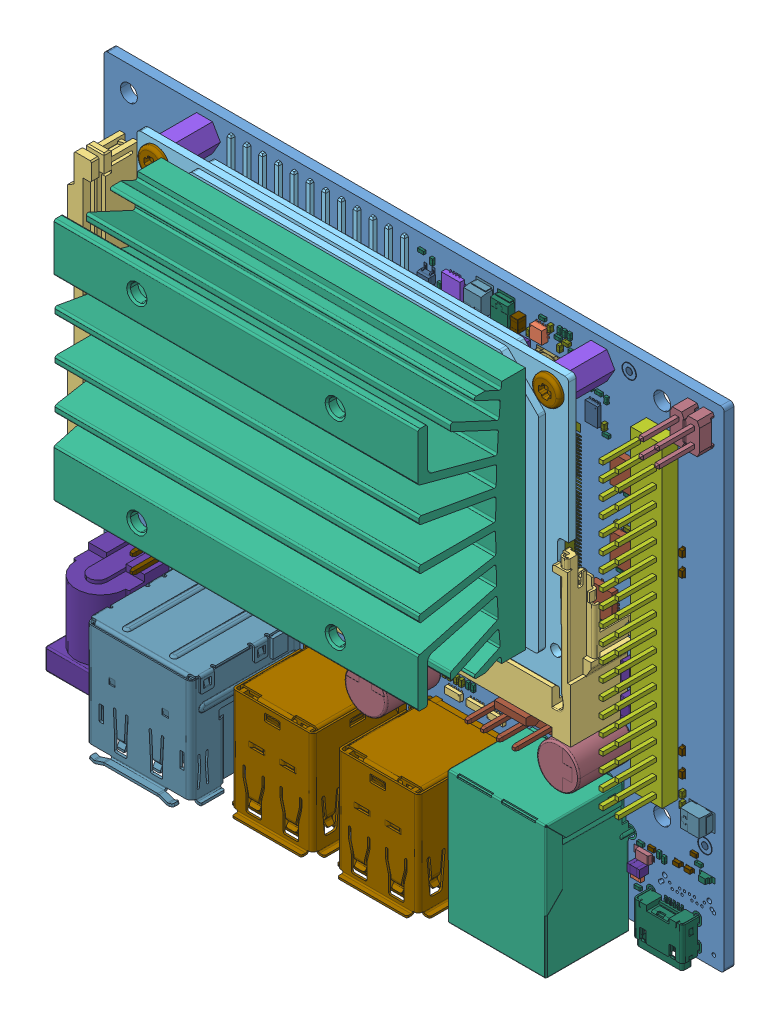
SolidWorks assembly Jetson_Nano_Dev_Kit_3D_b01, configuration Default. Lengths in mm. (continued)
Components (placement in the parent): (continued)
- Jetson_Nano_Dev_Kit_3D_b01(2)^Jetson_Nano_Dev_Kit_3D_b01-1: Jetson_Nano_Dev_Kit_3D_b01(2)^Jetson_Nano_Dev_Kit_3D_b01 [Default] at origin size (100 81.03 30.51) (virtual) (continued)
  - 642-13450_PORG_SYS_BOM^Jetson_Nano_Dev_Kit_3D_b01(2)_Jetson_Nano_Dev_Kit_3D_b01-1: 642-13450_PORG_SYS_BOM^Jetson_Nano_Dev_Kit_3D_b01(2)_Jetson_Nano_Dev_Kit_3D_b01 [Default] at origin size (100 81.03 23.18) (virtual) (continued)
    - 699-13449_PORG_DEV_KIT_PCB_ASSY^642-13450_PORG_SYS_BOM_Jetson_Nano_Dev_Kit_3D_b01(2)_Jetson_Nano_Dev_Kit_3D_b01-1: 699-13449_PORG_DEV_KIT_PCB_ASSY^642-13450_PORG_SYS_BOM_Jetson_Nano_Dev_Kit_3D_b01(2)_Jetson_Nano_Dev_Kit_3D_b01 [Default] at origin size (100 81.03 23.18) (virtual) (continued)
      - 600-13449_PORG_DEV_KIT_PCB_ASSY^699-13449_PORG_DEV_KIT_PCB_ASSY_642-13450_PORG_SYS_BOM_Jetson_Nano_Dev_Kit_3D_b01(2)_Jetson_Nano_Dev_Kit_3D_b01-1: 600-13449_PORG_DEV_KIT_PCB_ASSY^699-13449_PORG_DEV_KIT_PCB_ASSY_642-13450_PORG_SYS_BOM_Jetson_Nano_Dev_Kit_3D_b01(2)_Jetson_Nano_Dev_Kit_3D_b01 [Default] at origin size (100 81.03 23.18) (virtual) (continued)
        - 142-13449-1000-B01-SKU0000^600-13449_PORG_DEV_KIT_PCB_ASSY_699-13449_PORG_DEV_KIT_PCB_ASSY_642-13450_PORG_SYS_BOM_Jetson_Nano_Dev_Kit_3D_b01(2)_Jetson_Nano_Dev_Kit_3D_b01-1: 142-13449-1000-B01-SKU0000^600-13449_PORG_DEV_KIT_PCB_ASSY_699-13449_PORG_DEV_KIT_PCB_ASSY_642-13450_PORG_SYS_BOM_Jetson_Nano_Dev_Kit_3D_b01(2)_Jetson_Nano_Dev_Kit_3D_b01 [Default] at origin size (100 81.03 23.18) (virtual) (continued)
          - 0402_H040^142-13449-1000-B01-SKU0000_600-13449_PORG_DEV_KIT_PCB_ASSY_699-13449_PORG_DEV_KIT_PCB_ASSY_642-13450_PORG_SYS_BOM_Jetson_Nano_Dev_Kit_3D_b01(2)_Jetson_Nano_Dev_Kit_3D_b01-129: 0402_H040^142-13449-1000-B01-SKU0000_600-13449_PORG_DEV_KIT_PCB_ASSY_699-13449_PORG_DEV_KIT_PCB_ASSY_642-13450_PORG_SYS_BOM_Jetson_Nano_Dev_Kit_3D_b01(2)_Jetson_Nano_Dev_Kit_3D_b01 [Default] at (14.35 51.2 1.57) size (1 0.5 0.4) (virtual)
          - 0402_H040^142-13449-1000-B01-SKU0000_600-13449_PORG_DEV_KIT_PCB_ASSY_699-13449_PORG_DEV_KIT_PCB_ASSY_642-13450_PORG_SYS_BOM_Jetson_Nano_Dev_Kit_3D_b01(2)_Jetson_Nano_Dev_Kit_3D_b01-130: 0402_H040^142-13449-1000-B01-SKU0000_600-13449_PORG_DEV_KIT_PCB_ASSY_699-13449_PORG_DEV_KIT_PCB_ASSY_642-13450_PORG_SYS_BOM_Jetson_Nano_Dev_Kit_3D_b01(2)_Jetson_Nano_Dev_Kit_3D_b01 [Default] at (52.65 51.2 1.57) x (0 -1 0) z (0 0 1) size (1 0.5 0.4) (virtual)
          - 0402_H040^142-13449-1000-B01-SKU0000_600-13449_PORG_DEV_KIT_PCB_ASSY_699-13449_PORG_DEV_KIT_PCB_ASSY_642-13450_PORG_SYS_BOM_Jetson_Nano_Dev_Kit_3D_b01(2)_Jetson_Nano_Dev_Kit_3D_b01-131: 0402_H040^142-13449-1000-B01-SKU0000_600-13449_PORG_DEV_KIT_PCB_ASSY_699-13449_PORG_DEV_KIT_PCB_ASSY_642-13450_PORG_SYS_BOM_Jetson_Nano_Dev_Kit_3D_b01(2)_Jetson_Nano_Dev_Kit_3D_b01 [Default] at (74.1 5.25 1.57) x (0 -1 0) z (0 0 1) size (1 0.5 0.4) (virtual)
          - 0402_H040^142-13449-1000-B01-SKU0000_600-13449_PORG_DEV_KIT_PCB_ASSY_699-13449_PORG_DEV_KIT_PCB_ASSY_642-13450_PORG_SYS_BOM_Jetson_Nano_Dev_Kit_3D_b01(2)_Jetson_Nano_Dev_Kit_3D_b01-132: 0402_H040^142-13449-1000-B01-SKU0000_600-13449_PORG_DEV_KIT_PCB_ASSY_699-13449_PORG_DEV_KIT_PCB_ASSY_642-13450_PORG_SYS_BOM_Jetson_Nano_Dev_Kit_3D_b01(2)_Jetson_Nano_Dev_Kit_3D_b01 [Default] at (57.5 51.15 1.57) x (0 -1 0) z (0 0 1) size (1 0.5 0.4) (virtual)
          - 0402_H040^142-13449-1000-B01-SKU0000_600-13449_PORG_DEV_KIT_PCB_ASSY_699-13449_PORG_DEV_KIT_PCB_ASSY_642-13450_PORG_SYS_BOM_Jetson_Nano_Dev_Kit_3D_b01(2)_Jetson_Nano_Dev_Kit_3D_b01-133: 0402_H040^142-13449-1000-B01-SKU0000_600-13449_PORG_DEV_KIT_PCB_ASSY_699-13449_PORG_DEV_KIT_PCB_ASSY_642-13450_PORG_SYS_BOM_Jetson_Nano_Dev_Kit_3D_b01(2)_Jetson_Nano_Dev_Kit_3D_b01 [Default] at (55.4 47.8 1.57) x (0 -1 0) z (0 0 1) size (1 0.5 0.4) (virtual)
          - 0402_H040^142-13449-1000-B01-SKU0000_600-13449_PORG_DEV_KIT_PCB_ASSY_699-13449_PORG_DEV_KIT_PCB_ASSY_642-13450_PORG_SYS_BOM_Jetson_Nano_Dev_Kit_3D_b01(2)_Jetson_Nano_Dev_Kit_3D_b01-134: 0402_H040^142-13449-1000-B01-SKU0000_600-13449_PORG_DEV_KIT_PCB_ASSY_699-13449_PORG_DEV_KIT_PCB_ASSY_642-13450_PORG_SYS_BOM_Jetson_Nano_Dev_Kit_3D_b01(2)_Jetson_Nano_Dev_Kit_3D_b01 [Default] at (57.5 49.4 1.57) x (0 -1 0) z (0 0 1) size (1 0.5 0.4) (virtual)
          - 064-0377-000_2^142-13449-1000-B01-SKU0000_600-13449_PORG_DEV_KIT_PCB_ASSY_699-13449_PORG_DEV_KIT_PCB_ASSY_642-13450_PORG_SYS_BOM_Jetson_Nano_Dev_Kit_3D_b01(2)_Jetson_Nano_Dev_Kit_3D_b01-1: 064-0377-000_2^142-13449-1000-B01-SKU0000_600-13449_PORG_DEV_KIT_PCB_ASSY_699-13449_PORG_DEV_KIT_PCB_ASSY_642-13450_PORG_SYS_BOM_Jetson_Nano_Dev_Kit_3D_b01(2)_Jetson_Nano_Dev_Kit_3D_b01 [Default] at (2 -4.75 1.57) x (0 -1 0) z (0 0 1) size (14.64 10.09 14.5) (virtual)
          - 074-0117-000_2^142-13449-1000-B01-SKU0000_600-13449_PORG_DEV_KIT_PCB_ASSY_699-13449_PORG_DEV_KIT_PCB_ASSY_642-13450_PORG_SYS_BOM_Jetson_Nano_Dev_Kit_3D_b01(2)_Jetson_Nano_Dev_Kit_3D_b01-1: 074-0117-000_2^142-13449-1000-B01-SKU0000_600-13449_PORG_DEV_KIT_PCB_ASSY_699-13449_PORG_DEV_KIT_PCB_ASSY_642-13450_PORG_SYS_BOM_Jetson_Nano_Dev_Kit_3D_b01(2)_Jetson_Nano_Dev_Kit_3D_b01 [Default] at (8.8 2.15 1.57) x (0 1 0) z (0 0 1) size (5.08 2.54 11.66) (virtual)
          - 090-0096-000_1^142-13449-1000-B01-SKU0000_600-13449_PORG_DEV_KIT_PCB_ASSY_699-13449_PORG_DEV_KIT_PCB_ASSY_642-13450_PORG_SYS_BOM_Jetson_Nano_Dev_Kit_3D_b01(2)_Jetson_Nano_Dev_Kit_3D_b01-1: 090-0096-000_1^142-13449-1000-B01-SKU0000_600-13449_PORG_DEV_KIT_PCB_ASSY_699-13449_PORG_DEV_KIT_PCB_ASSY_642-13450_PORG_SYS_BOM_Jetson_Nano_Dev_Kit_3D_b01(2)_Jetson_Nano_Dev_Kit_3D_b01 [Default] at (33.75 44.05 1.57) size (1.2 0.6 0.4) (virtual)
          - 090-0309-000_1^142-13449-1000-B01-SKU0000_600-13449_PORG_DEV_KIT_PCB_ASSY_699-13449_PORG_DEV_KIT_PCB_ASSY_642-13450_PORG_SYS_BOM_Jetson_Nano_Dev_Kit_3D_b01(2)_Jetson_Nano_Dev_Kit_3D_b01-1: 090-0309-000_1^142-13449-1000-B01-SKU0000_600-13449_PORG_DEV_KIT_PCB_ASSY_699-13449_PORG_DEV_KIT_PCB_ASSY_642-13450_PORG_SYS_BOM_Jetson_Nano_Dev_Kit_3D_b01(2)_Jetson_Nano_Dev_Kit_3D_b01 [Default] at (15.95 50.3 1.57) size (1.2 0.6 0.4) (virtual)
          - 090-0231-000_1^142-13449-1000-B01-SKU0000_600-13449_PORG_DEV_KIT_PCB_ASSY_699-13449_PORG_DEV_KIT_PCB_ASSY_642-13450_PORG_SYS_BOM_Jetson_Nano_Dev_Kit_3D_b01(2)_Jetson_Nano_Dev_Kit_3D_b01-1: 090-0231-000_1^142-13449-1000-B01-SKU0000_600-13449_PORG_DEV_KIT_PCB_ASSY_699-13449_PORG_DEV_KIT_PCB_ASSY_642-13450_PORG_SYS_BOM_Jetson_Nano_Dev_Kit_3D_b01(2)_Jetson_Nano_Dev_Kit_3D_b01 [Default] at (35.3 0.7 1.57) x (-1 0 0) z (0 0 1) size (2.5 1.55 0.55) (virtual)
          - 090-0231-000_1^142-13449-1000-B01-SKU0000_600-13449_PORG_DEV_KIT_PCB_ASSY_699-13449_PORG_DEV_KIT_PCB_ASSY_642-13450_PORG_SYS_BOM_Jetson_Nano_Dev_Kit_3D_b01(2)_Jetson_Nano_Dev_Kit_3D_b01-2: 090-0231-000_1^142-13449-1000-B01-SKU0000_600-13449_PORG_DEV_KIT_PCB_ASSY_699-13449_PORG_DEV_KIT_PCB_ASSY_642-13450_PORG_SYS_BOM_Jetson_Nano_Dev_Kit_3D_b01(2)_Jetson_Nano_Dev_Kit_3D_b01 [Default] at (52.75 0.7 1.57) x (-1 0 0) z (0 0 1) size (2.5 1.55 0.55) (virtual)
          - 090-0231-000_1^142-13449-1000-B01-SKU0000_600-13449_PORG_DEV_KIT_PCB_ASSY_699-13449_PORG_DEV_KIT_PCB_ASSY_642-13450_PORG_SYS_BOM_Jetson_Nano_Dev_Kit_3D_b01(2)_Jetson_Nano_Dev_Kit_3D_b01-3: 090-0231-000_1^142-13449-1000-B01-SKU0000_600-13449_PORG_DEV_KIT_PCB_ASSY_699-13449_PORG_DEV_KIT_PCB_ASSY_642-13450_PORG_SYS_BOM_Jetson_Nano_Dev_Kit_3D_b01(2)_Jetson_Nano_Dev_Kit_3D_b01 [Default] at (56.25 0.7 1.57) size (2.5 1.55 0.55) (virtual)
          - 090-0231-000_1^142-13449-1000-B01-SKU0000_600-13449_PORG_DEV_KIT_PCB_ASSY_699-13449_PORG_DEV_KIT_PCB_ASSY_642-13450_PORG_SYS_BOM_Jetson_Nano_Dev_Kit_3D_b01(2)_Jetson_Nano_Dev_Kit_3D_b01-4: 090-0231-000_1^142-13449-1000-B01-SKU0000_600-13449_PORG_DEV_KIT_PCB_ASSY_699-13449_PORG_DEV_KIT_PCB_ASSY_642-13450_PORG_SYS_BOM_Jetson_Nano_Dev_Kit_3D_b01(2)_Jetson_Nano_Dev_Kit_3D_b01 [Default] at (59.65 0.7 1.57) size (2.5 1.55 0.55) (virtual)
          - 090-0231-000_1^142-13449-1000-B01-SKU0000_600-13449_PORG_DEV_KIT_PCB_ASSY_699-13449_PORG_DEV_KIT_PCB_ASSY_642-13450_PORG_SYS_BOM_Jetson_Nano_Dev_Kit_3D_b01(2)_Jetson_Nano_Dev_Kit_3D_b01-5: 090-0231-000_1^142-13449-1000-B01-SKU0000_600-13449_PORG_DEV_KIT_PCB_ASSY_699-13449_PORG_DEV_KIT_PCB_ASSY_642-13450_PORG_SYS_BOM_Jetson_Nano_Dev_Kit_3D_b01(2)_Jetson_Nano_Dev_Kit_3D_b01 [Default] at (39.1 0.7 1.57) size (2.5 1.55 0.55) (virtual)
          - 090-0231-000_1^142-13449-1000-B01-SKU0000_600-13449_PORG_DEV_KIT_PCB_ASSY_699-13449_PORG_DEV_KIT_PCB_ASSY_642-13450_PORG_SYS_BOM_Jetson_Nano_Dev_Kit_3D_b01(2)_Jetson_Nano_Dev_Kit_3D_b01-6: 090-0231-000_1^142-13449-1000-B01-SKU0000_600-13449_PORG_DEV_KIT_PCB_ASSY_699-13449_PORG_DEV_KIT_PCB_ASSY_642-13450_PORG_SYS_BOM_Jetson_Nano_Dev_Kit_3D_b01(2)_Jetson_Nano_Dev_Kit_3D_b01 [Default] at (42.15 0.7 1.57) size (2.5 1.55 0.55) (virtual)
          - 090-0296-000_2^142-13449-1000-B01-SKU0000_600-13449_PORG_DEV_KIT_PCB_ASSY_699-13449_PORG_DEV_KIT_PCB_ASSY_642-13450_PORG_SYS_BOM_Jetson_Nano_Dev_Kit_3D_b01(2)_Jetson_Nano_Dev_Kit_3D_b01-1: 090-0296-000_2^142-13449-1000-B01-SKU0000_600-13449_PORG_DEV_KIT_PCB_ASSY_699-13449_PORG_DEV_KIT_PCB_ASSY_642-13450_PORG_SYS_BOM_Jetson_Nano_Dev_Kit_3D_b01(2)_Jetson_Nano_Dev_Kit_3D_b01 [Default] at (14.6 1.8 1.57) size (2.5 1.55 0.55) (virtual)
          - 090-0296-000_2^142-13449-1000-B01-SKU0000_600-13449_PORG_DEV_KIT_PCB_ASSY_699-13449_PORG_DEV_KIT_PCB_ASSY_642-13450_PORG_SYS_BOM_Jetson_Nano_Dev_Kit_3D_b01(2)_Jetson_Nano_Dev_Kit_3D_b01-2: 090-0296-000_2^142-13449-1000-B01-SKU0000_600-13449_PORG_DEV_KIT_PCB_ASSY_699-13449_PORG_DEV_KIT_PCB_ASSY_642-13450_PORG_SYS_BOM_Jetson_Nano_Dev_Kit_3D_b01(2)_Jetson_Nano_Dev_Kit_3D_b01 [Default] at (19.1 1.8 1.57) size (2.5 1.55 0.55) (virtual)
          - 090-0231-000_1^142-13449-1000-B01-SKU0000_600-13449_PORG_DEV_KIT_PCB_ASSY_699-13449_PORG_DEV_KIT_PCB_ASSY_642-13450_PORG_SYS_BOM_Jetson_Nano_Dev_Kit_3D_b01(2)_Jetson_Nano_Dev_Kit_3D_b01-7: 090-0231-000_1^142-13449-1000-B01-SKU0000_600-13449_PORG_DEV_KIT_PCB_ASSY_699-13449_PORG_DEV_KIT_PCB_ASSY_642-13450_PORG_SYS_BOM_Jetson_Nano_Dev_Kit_3D_b01(2)_Jetson_Nano_Dev_Kit_3D_b01 [Default] at (22.5 1.4 1.57) size (2.5 1.55 0.55) (virtual)
          - 090-0231-000_1^142-13449-1000-B01-SKU0000_600-13449_PORG_DEV_KIT_PCB_ASSY_699-13449_PORG_DEV_KIT_PCB_ASSY_642-13450_PORG_SYS_BOM_Jetson_Nano_Dev_Kit_3D_b01(2)_Jetson_Nano_Dev_Kit_3D_b01-8: 090-0231-000_1^142-13449-1000-B01-SKU0000_600-13449_PORG_DEV_KIT_PCB_ASSY_699-13449_PORG_DEV_KIT_PCB_ASSY_642-13450_PORG_SYS_BOM_Jetson_Nano_Dev_Kit_3D_b01(2)_Jetson_Nano_Dev_Kit_3D_b01 [Default] at (28.45 3.35 1.57) size (2.5 1.55 0.55) (virtual)
          - 090-0231-000_1^142-13449-1000-B01-SKU0000_600-13449_PORG_DEV_KIT_PCB_ASSY_699-13449_PORG_DEV_KIT_PCB_ASSY_642-13450_PORG_SYS_BOM_Jetson_Nano_Dev_Kit_3D_b01(2)_Jetson_Nano_Dev_Kit_3D_b01-9: 090-0231-000_1^142-13449-1000-B01-SKU0000_600-13449_PORG_DEV_KIT_PCB_ASSY_699-13449_PORG_DEV_KIT_PCB_ASSY_642-13450_PORG_SYS_BOM_Jetson_Nano_Dev_Kit_3D_b01(2)_Jetson_Nano_Dev_Kit_3D_b01 [Default] at (31.65 3.35 1.57) size (2.5 1.55 0.55) (virtual)
          - LOGO_SILK_UL_ITE204896_I380_B^142-13449-1000-B01-SKU0000_600-13449_PORG_DEV_KIT_PCB_ASSY_699-13449_PORG_DEV_KIT_PCB_ASSY_642-13450_PORG_SYS_BOM_Jetson_Nano_Dev_Kit_3D_b01(2)_Jetson_Nano_Dev_Ki~-1: LOGO_SILK_UL_ITE204896_I380_B^142-13449-1000-B01-SKU0000_600-13449_PORG_DEV_KIT_PCB_ASSY_699-13449_PORG_DEV_KIT_PCB_ASSY_642-13450_PORG_SYS_BOM_Jetson_Nano_Dev_Kit_3D_b01(2)_Jetson_Nano_Dev_Ki~ [Default] at (57 5 0) x (-1 0 0) z (0 0 -1) size (13.08 8.6 0.05) (virtual)
          - LOGO_SILK_CE_I0175X0160^142-13449-1000-B01-SKU0000_600-13449_PORG_DEV_KIT_PCB_ASSY_699-13449_PORG_DEV_KIT_PCB_ASSY_642-13450_PORG_SYS_BOM_Jetson_Nano_Dev_Kit_3D_b01(2)_Jetson_Nano_Dev_Kit_3D_b~-1: LOGO_SILK_CE_I0175X0160^142-13449-1000-B01-SKU0000_600-13449_PORG_DEV_KIT_PCB_ASSY_699-13449_PORG_DEV_KIT_PCB_ASSY_642-13450_PORG_SYS_BOM_Jetson_Nano_Dev_Kit_3D_b01(2)_Jetson_Nano_Dev_Kit_3D_b~ [Default] at (39.9 5 0) x (-1 0 0) z (0 0 -1) size (4.55 3.29 0.05) (virtual)
          - LS_ICES_I0925X0040_CLASS_B^142-13449-1000-B01-SKU0000_600-13449_PORG_DEV_KIT_PCB_ASSY_699-13449_PORG_DEV_KIT_PCB_ASSY_642-13450_PORG_SYS_BOM_Jetson_Nano_Dev_Kit_3D_b01(2)_Jetson_Nano_Dev_Kit_3~-1: LS_ICES_I0925X0040_CLASS_B^142-13449-1000-B01-SKU0000_600-13449_PORG_DEV_KIT_PCB_ASSY_699-13449_PORG_DEV_KIT_PCB_ASSY_642-13450_PORG_SYS_BOM_Jetson_Nano_Dev_Kit_3D_b01(2)_Jetson_Nano_Dev_Kit_3~ [Default] at (53.35 28.2 0) x (-1 0 0) z (0 0 -1) size (17.94 1.42 0.03) (virtual)
          - 315-1062-000_1^142-13449-1000-B01-SKU0000_600-13449_PORG_DEV_KIT_PCB_ASSY_699-13449_PORG_DEV_KIT_PCB_ASSY_642-13450_PORG_SYS_BOM_Jetson_Nano_Dev_Kit_3D_b01(2)_Jetson_Nano_Dev_Kit_3D_b01-1: 315-1062-000_1^142-13449-1000-B01-SKU0000_600-13449_PORG_DEV_KIT_PCB_ASSY_699-13449_PORG_DEV_KIT_PCB_ASSY_642-13450_PORG_SYS_BOM_Jetson_Nano_Dev_Kit_3D_b01(2)_Jetson_Nano_Dev_Kit_3D_b01 [Default] at (5.4 8.95 1.57) x (0 1 0) z (0 0 1) size (3 3.58 1.45) (virtual)
          - 315-0620-000_1^142-13449-1000-B01-SKU0000_600-13449_PORG_DEV_KIT_PCB_ASSY_699-13449_PORG_DEV_KIT_PCB_ASSY_642-13450_PORG_SYS_BOM_Jetson_Nano_Dev_Kit_3D_b01(2)_Jetson_Nano_Dev_Kit_3D_b01-1: 315-0620-000_1^142-13449-1000-B01-SKU0000_600-13449_PORG_DEV_KIT_PCB_ASSY_699-13449_PORG_DEV_KIT_PCB_ASSY_642-13450_PORG_SYS_BOM_Jetson_Nano_Dev_Kit_3D_b01(2)_Jetson_Nano_Dev_Kit_3D_b01 [Default] at (60.1 51.8 1.57) x (-1 0 0) z (0 0 1) size (3 3.58 1.1) (virtual)
          - 315-1062-000_1^142-13449-1000-B01-SKU0000_600-13449_PORG_DEV_KIT_PCB_ASSY_699-13449_PORG_DEV_KIT_PCB_ASSY_642-13450_PORG_SYS_BOM_Jetson_Nano_Dev_Kit_3D_b01(2)_Jetson_Nano_Dev_Kit_3D_b01-2: 315-1062-000_1^142-13449-1000-B01-SKU0000_600-13449_PORG_DEV_KIT_PCB_ASSY_699-13449_PORG_DEV_KIT_PCB_ASSY_642-13450_PORG_SYS_BOM_Jetson_Nano_Dev_Kit_3D_b01(2)_Jetson_Nano_Dev_Kit_3D_b01 [Default] at (18 47.85 1.57) x (0 -1 0) z (0 0 1) size (3 3.58 1.45) (virtual)
          - 115-0138-000_1^142-13449-1000-B01-SKU0000_600-13449_PORG_DEV_KIT_PCB_ASSY_699-13449_PORG_DEV_KIT_PCB_ASSY_642-13450_PORG_SYS_BOM_Jetson_Nano_Dev_Kit_3D_b01(2)_Jetson_Nano_Dev_Kit_3D_b01-1: 115-0138-000_1^142-13449-1000-B01-SKU0000_600-13449_PORG_DEV_KIT_PCB_ASSY_699-13449_PORG_DEV_KIT_PCB_ASSY_642-13450_PORG_SYS_BOM_Jetson_Nano_Dev_Kit_3D_b01(2)_Jetson_Nano_Dev_Kit_3D_b01 [Default] at (48.55 56.85 1.57) size (2 2.88 1.1) (virtual)
          - 115-0138-000_1^142-13449-1000-B01-SKU0000_600-13449_PORG_DEV_KIT_PCB_ASSY_699-13449_PORG_DEV_KIT_PCB_ASSY_642-13450_PORG_SYS_BOM_Jetson_Nano_Dev_Kit_3D_b01(2)_Jetson_Nano_Dev_Kit_3D_b01-2: 115-0138-000_1^142-13449-1000-B01-SKU0000_600-13449_PORG_DEV_KIT_PCB_ASSY_699-13449_PORG_DEV_KIT_PCB_ASSY_642-13450_PORG_SYS_BOM_Jetson_Nano_Dev_Kit_3D_b01(2)_Jetson_Nano_Dev_Kit_3D_b01 [Default] at (59.25 23.15 1.57) size (2 2.88 1.1) (virtual)
          - 115-0138-000_1^142-13449-1000-B01-SKU0000_600-13449_PORG_DEV_KIT_PCB_ASSY_699-13449_PORG_DEV_KIT_PCB_ASSY_642-13450_PORG_SYS_BOM_Jetson_Nano_Dev_Kit_3D_b01(2)_Jetson_Nano_Dev_Kit_3D_b01-3: 115-0138-000_1^142-13449-1000-B01-SKU0000_600-13449_PORG_DEV_KIT_PCB_ASSY_699-13449_PORG_DEV_KIT_PCB_ASSY_642-13450_PORG_SYS_BOM_Jetson_Nano_Dev_Kit_3D_b01(2)_Jetson_Nano_Dev_Kit_3D_b01 [Default] at (28.15 46.45 1.57) x (0 -1 0) z (0 0 1) size (2 2.88 1.1) (virtual)
          - 115-1821-000_1^142-13449-1000-B01-SKU0000_600-13449_PORG_DEV_KIT_PCB_ASSY_699-13449_PORG_DEV_KIT_PCB_ASSY_642-13450_PORG_SYS_BOM_Jetson_Nano_Dev_Kit_3D_b01(2)_Jetson_Nano_Dev_Kit_3D_b01-1: 115-1821-000_1^142-13449-1000-B01-SKU0000_600-13449_PORG_DEV_KIT_PCB_ASSY_699-13449_PORG_DEV_KIT_PCB_ASSY_642-13450_PORG_SYS_BOM_Jetson_Nano_Dev_Kit_3D_b01(2)_Jetson_Nano_Dev_Kit_3D_b01 [Default] at (37.3 42.45 1.57) x (-1 0 0) z (0 0 1) size (2 2.88 1.1) (virtual)
          - 115-1821-000_1^142-13449-1000-B01-SKU0000_600-13449_PORG_DEV_KIT_PCB_ASSY_699-13449_PORG_DEV_KIT_PCB_ASSY_642-13450_PORG_SYS_BOM_Jetson_Nano_Dev_Kit_3D_b01(2)_Jetson_Nano_Dev_Kit_3D_b01-2: 115-1821-000_1^142-13449-1000-B01-SKU0000_600-13449_PORG_DEV_KIT_PCB_ASSY_699-13449_PORG_DEV_KIT_PCB_ASSY_642-13450_PORG_SYS_BOM_Jetson_Nano_Dev_Kit_3D_b01(2)_Jetson_Nano_Dev_Kit_3D_b01 [Default] at (31.2 48.35 1.57) size (2 2.88 1.1) (virtual)
          - 115-0742-000_2^142-13449-1000-B01-SKU0000_600-13449_PORG_DEV_KIT_PCB_ASSY_699-13449_PORG_DEV_KIT_PCB_ASSY_642-13450_PORG_SYS_BOM_Jetson_Nano_Dev_Kit_3D_b01(2)_Jetson_Nano_Dev_Kit_3D_b01-1: 115-0742-000_2^142-13449-1000-B01-SKU0000_600-13449_PORG_DEV_KIT_PCB_ASSY_699-13449_PORG_DEV_KIT_PCB_ASSY_642-13450_PORG_SYS_BOM_Jetson_Nano_Dev_Kit_3D_b01(2)_Jetson_Nano_Dev_Kit_3D_b01 [Default] at (33.85 46.4 1.57) size (2 2.88 1.1) (virtual)
          - 115-0742-000_2^142-13449-1000-B01-SKU0000_600-13449_PORG_DEV_KIT_PCB_ASSY_699-13449_PORG_DEV_KIT_PCB_ASSY_642-13450_PORG_SYS_BOM_Jetson_Nano_Dev_Kit_3D_b01(2)_Jetson_Nano_Dev_Kit_3D_b01-2: 115-0742-000_2^142-13449-1000-B01-SKU0000_600-13449_PORG_DEV_KIT_PCB_ASSY_699-13449_PORG_DEV_KIT_PCB_ASSY_642-13450_PORG_SYS_BOM_Jetson_Nano_Dev_Kit_3D_b01(2)_Jetson_Nano_Dev_Kit_3D_b01 [Default] at (36.35 46.9 1.57) x (-1 0 0) z (0 0 1) size (2 2.88 1.1) (virtual)
          - 091-0022-000_1^142-13449-1000-B01-SKU0000_600-13449_PORG_DEV_KIT_PCB_ASSY_699-13449_PORG_DEV_KIT_PCB_ASSY_642-13450_PORG_SYS_BOM_Jetson_Nano_Dev_Kit_3D_b01(2)_Jetson_Nano_Dev_Kit_3D_b01-1: 091-0022-000_1^142-13449-1000-B01-SKU0000_600-13449_PORG_DEV_KIT_PCB_ASSY_699-13449_PORG_DEV_KIT_PCB_ASSY_642-13450_PORG_SYS_BOM_Jetson_Nano_Dev_Kit_3D_b01(2)_Jetson_Nano_Dev_Kit_3D_b01 [Default] at (12.2 52 1.57) size (2 2.51 1.1) (virtual)
          - 091-0023-000_1^142-13449-1000-B01-SKU0000_600-13449_PORG_DEV_KIT_PCB_ASSY_699-13449_PORG_DEV_KIT_PCB_ASSY_642-13450_PORG_SYS_BOM_Jetson_Nano_Dev_Kit_3D_b01(2)_Jetson_Nano_Dev_Kit_3D_b01-1: 091-0023-000_1^142-13449-1000-B01-SKU0000_600-13449_PORG_DEV_KIT_PCB_ASSY_699-13449_PORG_DEV_KIT_PCB_ASSY_642-13450_PORG_SYS_BOM_Jetson_Nano_Dev_Kit_3D_b01(2)_Jetson_Nano_Dev_Kit_3D_b01 [Default] at (10.8 39.4 1.57) x (0 1 0) z (0 0 1) size (2 2.51 1.1) (virtual)
          - 080-1368-000_1^142-13449-1000-B01-SKU0000_600-13449_PORG_DEV_KIT_PCB_ASSY_699-13449_PORG_DEV_KIT_PCB_ASSY_642-13450_PORG_SYS_BOM_Jetson_Nano_Dev_Kit_3D_b01(2)_Jetson_Nano_Dev_Kit_3D_b01-1: 080-1368-000_1^142-13449-1000-B01-SKU0000_600-13449_PORG_DEV_KIT_PCB_ASSY_699-13449_PORG_DEV_KIT_PCB_ASSY_642-13450_PORG_SYS_BOM_Jetson_Nano_Dev_Kit_3D_b01(2)_Jetson_Nano_Dev_Kit_3D_b01 [Default] at (88 -14.3 1.57) size (8.9 7.2 4.46) (virtual)
          - LOGO_SILK_POSTAL_ADDRESS^142-13449-1000-B01-SKU0000_600-13449_PORG_DEV_KIT_PCB_ASSY_699-13449_PORG_DEV_KIT_PCB_ASSY_642-13450_PORG_SYS_BOM_Jetson_Nano_Dev_Kit_3D_b01(2)_Jetson_Nano_Dev_Kit_3D_~-1: LOGO_SILK_POSTAL_ADDRESS^142-13449-1000-B01-SKU0000_600-13449_PORG_DEV_KIT_PCB_ASSY_699-13449_PORG_DEV_KIT_PCB_ASSY_642-13450_PORG_SYS_BOM_Jetson_Nano_Dev_Kit_3D_b01(2)_Jetson_Nano_Dev_Kit_3D_~ [Default] at (61.35 31.2 0) x (-1 0 0) z (0 0 -1) size (18.11 2.17 0.05) (virtual)
          - LL_VENDOR_DATECODE_BOT_1R^142-13449-1000-B01-SKU0000_600-13449_PORG_DEV_KIT_PCB_ASSY_699-13449_PORG_DEV_KIT_PCB_ASSY_642-13450_PORG_SYS_BOM_Jetson_Nano_Dev_Kit_3D_b01(2)_Jetson_Nano_Dev_Kit_3D~-1: LL_VENDOR_DATECODE_BOT_1R^142-13449-1000-B01-SKU0000_600-13449_PORG_DEV_KIT_PCB_ASSY_699-13449_PORG_DEV_KIT_PCB_ASSY_642-13450_PORG_SYS_BOM_Jetson_Nano_Dev_Kit_3D_b01(2)_Jetson_Nano_Dev_Kit_3D~ [Default] at (-1.25 8.1 0) x (0 1 0) z (0 0 -1) size (35.76 2.49 0.07) (virtual)
          - 090-0172-000_1^142-13449-1000-B01-SKU0000_600-13449_PORG_DEV_KIT_PCB_ASSY_699-13449_PORG_DEV_KIT_PCB_ASSY_642-13450_PORG_SYS_BOM_Jetson_Nano_Dev_Kit_3D_b01(2)_Jetson_Nano_Dev_Kit_3D_b01-1: 090-0172-000_1^142-13449-1000-B01-SKU0000_600-13449_PORG_DEV_KIT_PCB_ASSY_699-13449_PORG_DEV_KIT_PCB_ASSY_642-13450_PORG_SYS_BOM_Jetson_Nano_Dev_Kit_3D_b01(2)_Jetson_Nano_Dev_Kit_3D_b01 [Default] at (69.9 23.45 1.57) x (0 1 0) z (0 0 1) size (1.41 0.61 0.55) (virtual)
          - 090-0172-000_1^142-13449-1000-B01-SKU0000_600-13449_PORG_DEV_KIT_PCB_ASSY_699-13449_PORG_DEV_KIT_PCB_ASSY_642-13450_PORG_SYS_BOM_Jetson_Nano_Dev_Kit_3D_b01(2)_Jetson_Nano_Dev_Kit_3D_b01-2: 090-0172-000_1^142-13449-1000-B01-SKU0000_600-13449_PORG_DEV_KIT_PCB_ASSY_699-13449_PORG_DEV_KIT_PCB_ASSY_642-13450_PORG_SYS_BOM_Jetson_Nano_Dev_Kit_3D_b01(2)_Jetson_Nano_Dev_Kit_3D_b01 [Default] at (71.4 23.45 1.57) x (0 1 0) z (0 0 1) size (1.41 0.61 0.55) (virtual)
          - 090-0172-000_1^142-13449-1000-B01-SKU0000_600-13449_PORG_DEV_KIT_PCB_ASSY_699-13449_PORG_DEV_KIT_PCB_ASSY_642-13450_PORG_SYS_BOM_Jetson_Nano_Dev_Kit_3D_b01(2)_Jetson_Nano_Dev_Kit_3D_b01-3: 090-0172-000_1^142-13449-1000-B01-SKU0000_600-13449_PORG_DEV_KIT_PCB_ASSY_699-13449_PORG_DEV_KIT_PCB_ASSY_642-13450_PORG_SYS_BOM_Jetson_Nano_Dev_Kit_3D_b01(2)_Jetson_Nano_Dev_Kit_3D_b01 [Default] at (5.3 21.25 1.57) x (0 -1 0) z (0 0 1) size (1.41 0.61 0.55) (virtual)
          - 090-0172-000_1^142-13449-1000-B01-SKU0000_600-13449_PORG_DEV_KIT_PCB_ASSY_699-13449_PORG_DEV_KIT_PCB_ASSY_642-13450_PORG_SYS_BOM_Jetson_Nano_Dev_Kit_3D_b01(2)_Jetson_Nano_Dev_Kit_3D_b01-4: 090-0172-000_1^142-13449-1000-B01-SKU0000_600-13449_PORG_DEV_KIT_PCB_ASSY_699-13449_PORG_DEV_KIT_PCB_ASSY_642-13450_PORG_SYS_BOM_Jetson_Nano_Dev_Kit_3D_b01(2)_Jetson_Nano_Dev_Kit_3D_b01 [Default] at (4.1 22.55 1.57) x (0 1 0) z (0 0 1) size (1.41 0.61 0.55) (virtual)
          - 090-0172-000_1^142-13449-1000-B01-SKU0000_600-13449_PORG_DEV_KIT_PCB_ASSY_699-13449_PORG_DEV_KIT_PCB_ASSY_642-13450_PORG_SYS_BOM_Jetson_Nano_Dev_Kit_3D_b01(2)_Jetson_Nano_Dev_Kit_3D_b01-5: 090-0172-000_1^142-13449-1000-B01-SKU0000_600-13449_PORG_DEV_KIT_PCB_ASSY_699-13449_PORG_DEV_KIT_PCB_ASSY_642-13450_PORG_SYS_BOM_Jetson_Nano_Dev_Kit_3D_b01(2)_Jetson_Nano_Dev_Kit_3D_b01 [Default] at (5 44.55 1.57) x (0 -1 0) z (0 0 1) size (1.41 0.61 0.55) (virtual)
          - 090-0172-000_1^142-13449-1000-B01-SKU0000_600-13449_PORG_DEV_KIT_PCB_ASSY_699-13449_PORG_DEV_KIT_PCB_ASSY_642-13450_PORG_SYS_BOM_Jetson_Nano_Dev_Kit_3D_b01(2)_Jetson_Nano_Dev_Kit_3D_b01-6: 090-0172-000_1^142-13449-1000-B01-SKU0000_600-13449_PORG_DEV_KIT_PCB_ASSY_699-13449_PORG_DEV_KIT_PCB_ASSY_642-13450_PORG_SYS_BOM_Jetson_Nano_Dev_Kit_3D_b01(2)_Jetson_Nano_Dev_Kit_3D_b01 [Default] at (5 46.35 1.57) x (0 1 0) z (0 0 1) size (1.41 0.61 0.55) (virtual)
          - 090-0172-000_1^142-13449-1000-B01-SKU0000_600-13449_PORG_DEV_KIT_PCB_ASSY_699-13449_PORG_DEV_KIT_PCB_ASSY_642-13450_PORG_SYS_BOM_Jetson_Nano_Dev_Kit_3D_b01(2)_Jetson_Nano_Dev_Kit_3D_b01-7: 090-0172-000_1^142-13449-1000-B01-SKU0000_600-13449_PORG_DEV_KIT_PCB_ASSY_699-13449_PORG_DEV_KIT_PCB_ASSY_642-13450_PORG_SYS_BOM_Jetson_Nano_Dev_Kit_3D_b01(2)_Jetson_Nano_Dev_Kit_3D_b01 [Default] at (3.95 43.4 1.57) x (0 1 0) z (0 0 1) size (1.41 0.61 0.55) (virtual)
          - 090-0172-000_1^142-13449-1000-B01-SKU0000_600-13449_PORG_DEV_KIT_PCB_ASSY_699-13449_PORG_DEV_KIT_PCB_ASSY_642-13450_PORG_SYS_BOM_Jetson_Nano_Dev_Kit_3D_b01(2)_Jetson_Nano_Dev_Kit_3D_b01-8: 090-0172-000_1^142-13449-1000-B01-SKU0000_600-13449_PORG_DEV_KIT_PCB_ASSY_699-13449_PORG_DEV_KIT_PCB_ASSY_642-13450_PORG_SYS_BOM_Jetson_Nano_Dev_Kit_3D_b01(2)_Jetson_Nano_Dev_Kit_3D_b01 [Default] at (3.95 19.9 1.57) x (0 1 0) z (0 0 1) size (1.41 0.61 0.55) (virtual)
          - 090-0172-000_1^142-13449-1000-B01-SKU0000_600-13449_PORG_DEV_KIT_PCB_ASSY_699-13449_PORG_DEV_KIT_PCB_ASSY_642-13450_PORG_SYS_BOM_Jetson_Nano_Dev_Kit_3D_b01(2)_Jetson_Nano_Dev_Kit_3D_b01-9: 090-0172-000_1^142-13449-1000-B01-SKU0000_600-13449_PORG_DEV_KIT_PCB_ASSY_699-13449_PORG_DEV_KIT_PCB_ASSY_642-13450_PORG_SYS_BOM_Jetson_Nano_Dev_Kit_3D_b01(2)_Jetson_Nano_Dev_Kit_3D_b01 [Default] at (3.95 41.6 1.57) x (0 -1 0) z (0 0 1) size (1.41 0.61 0.55) (virtual)
          - 090-0172-000_1^142-13449-1000-B01-SKU0000_600-13449_PORG_DEV_KIT_PCB_ASSY_699-13449_PORG_DEV_KIT_PCB_ASSY_642-13450_PORG_SYS_BOM_Jetson_Nano_Dev_Kit_3D_b01(2)_Jetson_Nano_Dev_Kit_3D_b01-10: 090-0172-000_1^142-13449-1000-B01-SKU0000_600-13449_PORG_DEV_KIT_PCB_ASSY_699-13449_PORG_DEV_KIT_PCB_ASSY_642-13450_PORG_SYS_BOM_Jetson_Nano_Dev_Kit_3D_b01(2)_Jetson_Nano_Dev_Kit_3D_b01 [Default] at (3.95 18.1 1.57) x (0 -1 0) z (0 0 1) size (1.41 0.61 0.55) (virtual)
          - 090-0172-000_1^142-13449-1000-B01-SKU0000_600-13449_PORG_DEV_KIT_PCB_ASSY_699-13449_PORG_DEV_KIT_PCB_ASSY_642-13450_PORG_SYS_BOM_Jetson_Nano_Dev_Kit_3D_b01(2)_Jetson_Nano_Dev_Kit_3D_b01-11: 090-0172-000_1^142-13449-1000-B01-SKU0000_600-13449_PORG_DEV_KIT_PCB_ASSY_699-13449_PORG_DEV_KIT_PCB_ASSY_642-13450_PORG_SYS_BOM_Jetson_Nano_Dev_Kit_3D_b01(2)_Jetson_Nano_Dev_Kit_3D_b01 [Default] at (4.35 40.15 1.57) size (1.41 0.61 0.55) (virtual)
          - 090-0172-000_1^142-13449-1000-B01-SKU0000_600-13449_PORG_DEV_KIT_PCB_ASSY_699-13449_PORG_DEV_KIT_PCB_ASSY_642-13450_PORG_SYS_BOM_Jetson_Nano_Dev_Kit_3D_b01(2)_Jetson_Nano_Dev_Kit_3D_b01-12: 090-0172-000_1^142-13449-1000-B01-SKU0000_600-13449_PORG_DEV_KIT_PCB_ASSY_699-13449_PORG_DEV_KIT_PCB_ASSY_642-13450_PORG_SYS_BOM_Jetson_Nano_Dev_Kit_3D_b01(2)_Jetson_Nano_Dev_Kit_3D_b01 [Default] at (3.95 16.3 1.57) x (0 1 0) z (0 0 1) size (1.41 0.61 0.55) (virtual)
          - 090-0172-000_1^142-13449-1000-B01-SKU0000_600-13449_PORG_DEV_KIT_PCB_ASSY_699-13449_PORG_DEV_KIT_PCB_ASSY_642-13450_PORG_SYS_BOM_Jetson_Nano_Dev_Kit_3D_b01(2)_Jetson_Nano_Dev_Kit_3D_b01-13: 090-0172-000_1^142-13449-1000-B01-SKU0000_600-13449_PORG_DEV_KIT_PCB_ASSY_699-13449_PORG_DEV_KIT_PCB_ASSY_642-13450_PORG_SYS_BOM_Jetson_Nano_Dev_Kit_3D_b01(2)_Jetson_Nano_Dev_Kit_3D_b01 [Default] at (4.35 38.8 1.57) size (1.41 0.61 0.55) (virtual)
          - 090-0172-000_1^142-13449-1000-B01-SKU0000_600-13449_PORG_DEV_KIT_PCB_ASSY_699-13449_PORG_DEV_KIT_PCB_ASSY_642-13450_PORG_SYS_BOM_Jetson_Nano_Dev_Kit_3D_b01(2)_Jetson_Nano_Dev_Kit_3D_b01-14: 090-0172-000_1^142-13449-1000-B01-SKU0000_600-13449_PORG_DEV_KIT_PCB_ASSY_699-13449_PORG_DEV_KIT_PCB_ASSY_642-13450_PORG_SYS_BOM_Jetson_Nano_Dev_Kit_3D_b01(2)_Jetson_Nano_Dev_Kit_3D_b01 [Default] at (3.95 14.5 1.57) x (0 -1 0) z (0 0 1) size (1.41 0.61 0.55) (virtual)
          - 090-0172-000_1^142-13449-1000-B01-SKU0000_600-13449_PORG_DEV_KIT_PCB_ASSY_699-13449_PORG_DEV_KIT_PCB_ASSY_642-13450_PORG_SYS_BOM_Jetson_Nano_Dev_Kit_3D_b01(2)_Jetson_Nano_Dev_Kit_3D_b01-15: 090-0172-000_1^142-13449-1000-B01-SKU0000_600-13449_PORG_DEV_KIT_PCB_ASSY_699-13449_PORG_DEV_KIT_PCB_ASSY_642-13450_PORG_SYS_BOM_Jetson_Nano_Dev_Kit_3D_b01(2)_Jetson_Nano_Dev_Kit_3D_b01 [Default] at (3.95 37 1.57) x (0 1 0) z (0 0 1) size (1.41 0.61 0.55) (virtual)
          - 090-0172-000_1^142-13449-1000-B01-SKU0000_600-13449_PORG_DEV_KIT_PCB_ASSY_699-13449_PORG_DEV_KIT_PCB_ASSY_642-13450_PORG_SYS_BOM_Jetson_Nano_Dev_Kit_3D_b01(2)_Jetson_Nano_Dev_Kit_3D_b01-16: 090-0172-000_1^142-13449-1000-B01-SKU0000_600-13449_PORG_DEV_KIT_PCB_ASSY_699-13449_PORG_DEV_KIT_PCB_ASSY_642-13450_PORG_SYS_BOM_Jetson_Nano_Dev_Kit_3D_b01(2)_Jetson_Nano_Dev_Kit_3D_b01 [Default] at (4.35 13.05 1.57) size (1.41 0.61 0.55) (virtual)
          - 090-0172-000_1^142-13449-1000-B01-SKU0000_600-13449_PORG_DEV_KIT_PCB_ASSY_699-13449_PORG_DEV_KIT_PCB_ASSY_642-13450_PORG_SYS_BOM_Jetson_Nano_Dev_Kit_3D_b01(2)_Jetson_Nano_Dev_Kit_3D_b01-17: 090-0172-000_1^142-13449-1000-B01-SKU0000_600-13449_PORG_DEV_KIT_PCB_ASSY_699-13449_PORG_DEV_KIT_PCB_ASSY_642-13450_PORG_SYS_BOM_Jetson_Nano_Dev_Kit_3D_b01(2)_Jetson_Nano_Dev_Kit_3D_b01 [Default] at (3.95 35.2 1.57) x (0 -1 0) z (0 0 1) size (1.41 0.61 0.55) (virtual)
          - 090-0172-000_1^142-13449-1000-B01-SKU0000_600-13449_PORG_DEV_KIT_PCB_ASSY_699-13449_PORG_DEV_KIT_PCB_ASSY_642-13450_PORG_SYS_BOM_Jetson_Nano_Dev_Kit_3D_b01(2)_Jetson_Nano_Dev_Kit_3D_b01-18: 090-0172-000_1^142-13449-1000-B01-SKU0000_600-13449_PORG_DEV_KIT_PCB_ASSY_699-13449_PORG_DEV_KIT_PCB_ASSY_642-13450_PORG_SYS_BOM_Jetson_Nano_Dev_Kit_3D_b01(2)_Jetson_Nano_Dev_Kit_3D_b01 [Default] at (4.35 11.8 1.57) size (1.41 0.61 0.55) (virtual)
          - 090-0243-000_1^142-13449-1000-B01-SKU0000_600-13449_PORG_DEV_KIT_PCB_ASSY_699-13449_PORG_DEV_KIT_PCB_ASSY_642-13450_PORG_SYS_BOM_Jetson_Nano_Dev_Kit_3D_b01(2)_Jetson_Nano_Dev_Kit_3D_b01-1: 090-0243-000_1^142-13449-1000-B01-SKU0000_600-13449_PORG_DEV_KIT_PCB_ASSY_699-13449_PORG_DEV_KIT_PCB_ASSY_642-13450_PORG_SYS_BOM_Jetson_Nano_Dev_Kit_3D_b01(2)_Jetson_Nano_Dev_Kit_3D_b01 [Default] at (42.275 49.45 1.57) size (1.41 0.61 0.45) (virtual)
          - 090-0243-000_1^142-13449-1000-B01-SKU0000_600-13449_PORG_DEV_KIT_PCB_ASSY_699-13449_PORG_DEV_KIT_PCB_ASSY_642-13450_PORG_SYS_BOM_Jetson_Nano_Dev_Kit_3D_b01(2)_Jetson_Nano_Dev_Kit_3D_b01-2: 090-0243-000_1^142-13449-1000-B01-SKU0000_600-13449_PORG_DEV_KIT_PCB_ASSY_699-13449_PORG_DEV_KIT_PCB_ASSY_642-13450_PORG_SYS_BOM_Jetson_Nano_Dev_Kit_3D_b01(2)_Jetson_Nano_Dev_Kit_3D_b01 [Default] at (40.375 49.45 1.57) x (-1 0 0) z (0 0 1) size (1.41 0.61 0.45) (virtual)
          - 090-0243-000_1^142-13449-1000-B01-SKU0000_600-13449_PORG_DEV_KIT_PCB_ASSY_699-13449_PORG_DEV_KIT_PCB_ASSY_642-13450_PORG_SYS_BOM_Jetson_Nano_Dev_Kit_3D_b01(2)_Jetson_Nano_Dev_Kit_3D_b01-3: 090-0243-000_1^142-13449-1000-B01-SKU0000_600-13449_PORG_DEV_KIT_PCB_ASSY_699-13449_PORG_DEV_KIT_PCB_ASSY_642-13450_PORG_SYS_BOM_Jetson_Nano_Dev_Kit_3D_b01(2)_Jetson_Nano_Dev_Kit_3D_b01 [Default] at (11.1 1.7 1.57) x (0 -1 0) z (0 0 1) size (1.41 0.61 0.45) (virtual)
          - 090-0243-000_1^142-13449-1000-B01-SKU0000_600-13449_PORG_DEV_KIT_PCB_ASSY_699-13449_PORG_DEV_KIT_PCB_ASSY_642-13450_PORG_SYS_BOM_Jetson_Nano_Dev_Kit_3D_b01(2)_Jetson_Nano_Dev_Kit_3D_b01-4: 090-0243-000_1^142-13449-1000-B01-SKU0000_600-13449_PORG_DEV_KIT_PCB_ASSY_699-13449_PORG_DEV_KIT_PCB_ASSY_642-13450_PORG_SYS_BOM_Jetson_Nano_Dev_Kit_3D_b01(2)_Jetson_Nano_Dev_Kit_3D_b01 [Default] at (36.15 49.45 1.57) size (1.41 0.61 0.45) (virtual)
          - 090-0243-000_1^142-13449-1000-B01-SKU0000_600-13449_PORG_DEV_KIT_PCB_ASSY_699-13449_PORG_DEV_KIT_PCB_ASSY_642-13450_PORG_SYS_BOM_Jetson_Nano_Dev_Kit_3D_b01(2)_Jetson_Nano_Dev_Kit_3D_b01-5: 090-0243-000_1^142-13449-1000-B01-SKU0000_600-13449_PORG_DEV_KIT_PCB_ASSY_699-13449_PORG_DEV_KIT_PCB_ASSY_642-13450_PORG_SYS_BOM_Jetson_Nano_Dev_Kit_3D_b01(2)_Jetson_Nano_Dev_Kit_3D_b01 [Default] at (21.35 49.45 1.57) size (1.41 0.61 0.45) (virtual)
          - 090-0243-000_1^142-13449-1000-B01-SKU0000_600-13449_PORG_DEV_KIT_PCB_ASSY_699-13449_PORG_DEV_KIT_PCB_ASSY_642-13450_PORG_SYS_BOM_Jetson_Nano_Dev_Kit_3D_b01(2)_Jetson_Nano_Dev_Kit_3D_b01-6: 090-0243-000_1^142-13449-1000-B01-SKU0000_600-13449_PORG_DEV_KIT_PCB_ASSY_699-13449_PORG_DEV_KIT_PCB_ASSY_642-13450_PORG_SYS_BOM_Jetson_Nano_Dev_Kit_3D_b01(2)_Jetson_Nano_Dev_Kit_3D_b01 [Default] at (34.3 49.45 1.57) size (1.41 0.61 0.45) (virtual)
          - 090-0243-000_1^142-13449-1000-B01-SKU0000_600-13449_PORG_DEV_KIT_PCB_ASSY_699-13449_PORG_DEV_KIT_PCB_ASSY_642-13450_PORG_SYS_BOM_Jetson_Nano_Dev_Kit_3D_b01(2)_Jetson_Nano_Dev_Kit_3D_b01-7: 090-0243-000_1^142-13449-1000-B01-SKU0000_600-13449_PORG_DEV_KIT_PCB_ASSY_699-13449_PORG_DEV_KIT_PCB_ASSY_642-13450_PORG_SYS_BOM_Jetson_Nano_Dev_Kit_3D_b01(2)_Jetson_Nano_Dev_Kit_3D_b01 [Default] at (23.15 49.45 1.57) x (-1 0 0) z (0 0 1) size (1.41 0.61 0.45) (virtual)
          - 090-0243-000_1^142-13449-1000-B01-SKU0000_600-13449_PORG_DEV_KIT_PCB_ASSY_699-13449_PORG_DEV_KIT_PCB_ASSY_642-13450_PORG_SYS_BOM_Jetson_Nano_Dev_Kit_3D_b01(2)_Jetson_Nano_Dev_Kit_3D_b01-8: 090-0243-000_1^142-13449-1000-B01-SKU0000_600-13449_PORG_DEV_KIT_PCB_ASSY_699-13449_PORG_DEV_KIT_PCB_ASSY_642-13450_PORG_SYS_BOM_Jetson_Nano_Dev_Kit_3D_b01(2)_Jetson_Nano_Dev_Kit_3D_b01 [Default] at (27.95 49.45 1.57) size (1.41 0.61 0.45) (virtual)
          - 090-0172-000_1^142-13449-1000-B01-SKU0000_600-13449_PORG_DEV_KIT_PCB_ASSY_699-13449_PORG_DEV_KIT_PCB_ASSY_642-13450_PORG_SYS_BOM_Jetson_Nano_Dev_Kit_3D_b01(2)_Jetson_Nano_Dev_Kit_3D_b01-19: 090-0172-000_1^142-13449-1000-B01-SKU0000_600-13449_PORG_DEV_KIT_PCB_ASSY_699-13449_PORG_DEV_KIT_PCB_ASSY_642-13450_PORG_SYS_BOM_Jetson_Nano_Dev_Kit_3D_b01(2)_Jetson_Nano_Dev_Kit_3D_b01 [Default] at (89.55 7.85 1.57) x (0 1 0) z (0 0 1) size (1.41 0.61 0.55) (virtual)
          - 090-0172-000_1^142-13449-1000-B01-SKU0000_600-13449_PORG_DEV_KIT_PCB_ASSY_699-13449_PORG_DEV_KIT_PCB_ASSY_642-13450_PORG_SYS_BOM_Jetson_Nano_Dev_Kit_3D_b01(2)_Jetson_Nano_Dev_Kit_3D_b01-20: 090-0172-000_1^142-13449-1000-B01-SKU0000_600-13449_PORG_DEV_KIT_PCB_ASSY_699-13449_PORG_DEV_KIT_PCB_ASSY_642-13450_PORG_SYS_BOM_Jetson_Nano_Dev_Kit_3D_b01(2)_Jetson_Nano_Dev_Kit_3D_b01 [Default] at (89.55 11.05 1.57) x (0 1 0) z (0 0 1) size (1.41 0.61 0.55) (virtual)
          - 090-0172-000_1^142-13449-1000-B01-SKU0000_600-13449_PORG_DEV_KIT_PCB_ASSY_699-13449_PORG_DEV_KIT_PCB_ASSY_642-13450_PORG_SYS_BOM_Jetson_Nano_Dev_Kit_3D_b01(2)_Jetson_Nano_Dev_Kit_3D_b01-21: 090-0172-000_1^142-13449-1000-B01-SKU0000_600-13449_PORG_DEV_KIT_PCB_ASSY_699-13449_PORG_DEV_KIT_PCB_ASSY_642-13450_PORG_SYS_BOM_Jetson_Nano_Dev_Kit_3D_b01(2)_Jetson_Nano_Dev_Kit_3D_b01 [Default] at (89.55 35.9 1.57) x (0 -1 0) z (0 0 1) size (1.41 0.61 0.55) (virtual)
          - 090-0172-000_1^142-13449-1000-B01-SKU0000_600-13449_PORG_DEV_KIT_PCB_ASSY_699-13449_PORG_DEV_KIT_PCB_ASSY_642-13450_PORG_SYS_BOM_Jetson_Nano_Dev_Kit_3D_b01(2)_Jetson_Nano_Dev_Kit_3D_b01-22: 090-0172-000_1^142-13449-1000-B01-SKU0000_600-13449_PORG_DEV_KIT_PCB_ASSY_699-13449_PORG_DEV_KIT_PCB_ASSY_642-13450_PORG_SYS_BOM_Jetson_Nano_Dev_Kit_3D_b01(2)_Jetson_Nano_Dev_Kit_3D_b01 [Default] at (89.55 38.75 1.57) x (0 1 0) z (0 0 1) size (1.41 0.61 0.55) (virtual)
          - 090-0243-000_1^142-13449-1000-B01-SKU0000_600-13449_PORG_DEV_KIT_PCB_ASSY_699-13449_PORG_DEV_KIT_PCB_ASSY_642-13450_PORG_SYS_BOM_Jetson_Nano_Dev_Kit_3D_b01(2)_Jetson_Nano_Dev_Kit_3D_b01-9: 090-0243-000_1^142-13449-1000-B01-SKU0000_600-13449_PORG_DEV_KIT_PCB_ASSY_699-13449_PORG_DEV_KIT_PCB_ASSY_642-13450_PORG_SYS_BOM_Jetson_Nano_Dev_Kit_3D_b01(2)_Jetson_Nano_Dev_Kit_3D_b01 [Default] at (8.35 -6.3 1.57) x (0 -1 0) z (0 0 1) size (1.41 0.61 0.45) (virtual)
          - 090-0172-000_1^142-13449-1000-B01-SKU0000_600-13449_PORG_DEV_KIT_PCB_ASSY_699-13449_PORG_DEV_KIT_PCB_ASSY_642-13450_PORG_SYS_BOM_Jetson_Nano_Dev_Kit_3D_b01(2)_Jetson_Nano_Dev_Kit_3D_b01-23: 090-0172-000_1^142-13449-1000-B01-SKU0000_600-13449_PORG_DEV_KIT_PCB_ASSY_699-13449_PORG_DEV_KIT_PCB_ASSY_642-13450_PORG_SYS_BOM_Jetson_Nano_Dev_Kit_3D_b01(2)_Jetson_Nano_Dev_Kit_3D_b01 [Default] at (9.75 -5.15 1.57) x (-1 0 0) z (0 0 1) size (1.41 0.61 0.55) (virtual)
          - 090-0172-000_1^142-13449-1000-B01-SKU0000_600-13449_PORG_DEV_KIT_PCB_ASSY_699-13449_PORG_DEV_KIT_PCB_ASSY_642-13450_PORG_SYS_BOM_Jetson_Nano_Dev_Kit_3D_b01(2)_Jetson_Nano_Dev_Kit_3D_b01-24: 090-0172-000_1^142-13449-1000-B01-SKU0000_600-13449_PORG_DEV_KIT_PCB_ASSY_699-13449_PORG_DEV_KIT_PCB_ASSY_642-13450_PORG_SYS_BOM_Jetson_Nano_Dev_Kit_3D_b01(2)_Jetson_Nano_Dev_Kit_3D_b01 [Default] at (10.05 -12.1 1.57) x (-1 0 0) z (0 0 1) size (1.41 0.61 0.55) (virtual)
          - 090-0243-000_1^142-13449-1000-B01-SKU0000_600-13449_PORG_DEV_KIT_PCB_ASSY_699-13449_PORG_DEV_KIT_PCB_ASSY_642-13450_PORG_SYS_BOM_Jetson_Nano_Dev_Kit_3D_b01(2)_Jetson_Nano_Dev_Kit_3D_b01-10: 090-0243-000_1^142-13449-1000-B01-SKU0000_600-13449_PORG_DEV_KIT_PCB_ASSY_699-13449_PORG_DEV_KIT_PCB_ASSY_642-13450_PORG_SYS_BOM_Jetson_Nano_Dev_Kit_3D_b01(2)_Jetson_Nano_Dev_Kit_3D_b01 [Default] at (9.8 -6.25 1.57) x (-1 0 0) z (0 0 1) size (1.41 0.61 0.45) (virtual)
          - 090-0243-000_1^142-13449-1000-B01-SKU0000_600-13449_PORG_DEV_KIT_PCB_ASSY_699-13449_PORG_DEV_KIT_PCB_ASSY_642-13450_PORG_SYS_BOM_Jetson_Nano_Dev_Kit_3D_b01(2)_Jetson_Nano_Dev_Kit_3D_b01-11: 090-0243-000_1^142-13449-1000-B01-SKU0000_600-13449_PORG_DEV_KIT_PCB_ASSY_699-13449_PORG_DEV_KIT_PCB_ASSY_642-13450_PORG_SYS_BOM_Jetson_Nano_Dev_Kit_3D_b01(2)_Jetson_Nano_Dev_Kit_3D_b01 [Default] at (8.85 -9.55 1.57) x (-1 0 0) z (0 0 1) size (1.41 0.61 0.45) (virtual)
          - 090-0172-000_1^142-13449-1000-B01-SKU0000_600-13449_PORG_DEV_KIT_PCB_ASSY_699-13449_PORG_DEV_KIT_PCB_ASSY_642-13450_PORG_SYS_BOM_Jetson_Nano_Dev_Kit_3D_b01(2)_Jetson_Nano_Dev_Kit_3D_b01-25: 090-0172-000_1^142-13449-1000-B01-SKU0000_600-13449_PORG_DEV_KIT_PCB_ASSY_699-13449_PORG_DEV_KIT_PCB_ASSY_642-13450_PORG_SYS_BOM_Jetson_Nano_Dev_Kit_3D_b01(2)_Jetson_Nano_Dev_Kit_3D_b01 [Default] at (90.6 -5 1.57) size (1.41 0.61 0.55) (virtual)
          - 090-0172-000_1^142-13449-1000-B01-SKU0000_600-13449_PORG_DEV_KIT_PCB_ASSY_699-13449_PORG_DEV_KIT_PCB_ASSY_642-13450_PORG_SYS_BOM_Jetson_Nano_Dev_Kit_3D_b01(2)_Jetson_Nano_Dev_Kit_3D_b01-26: 090-0172-000_1^142-13449-1000-B01-SKU0000_600-13449_PORG_DEV_KIT_PCB_ASSY_699-13449_PORG_DEV_KIT_PCB_ASSY_642-13450_PORG_SYS_BOM_Jetson_Nano_Dev_Kit_3D_b01(2)_Jetson_Nano_Dev_Kit_3D_b01 [Default] at (88.8 -5 1.57) x (-1 0 0) z (0 0 1) size (1.41 0.61 0.55) (virtual)
